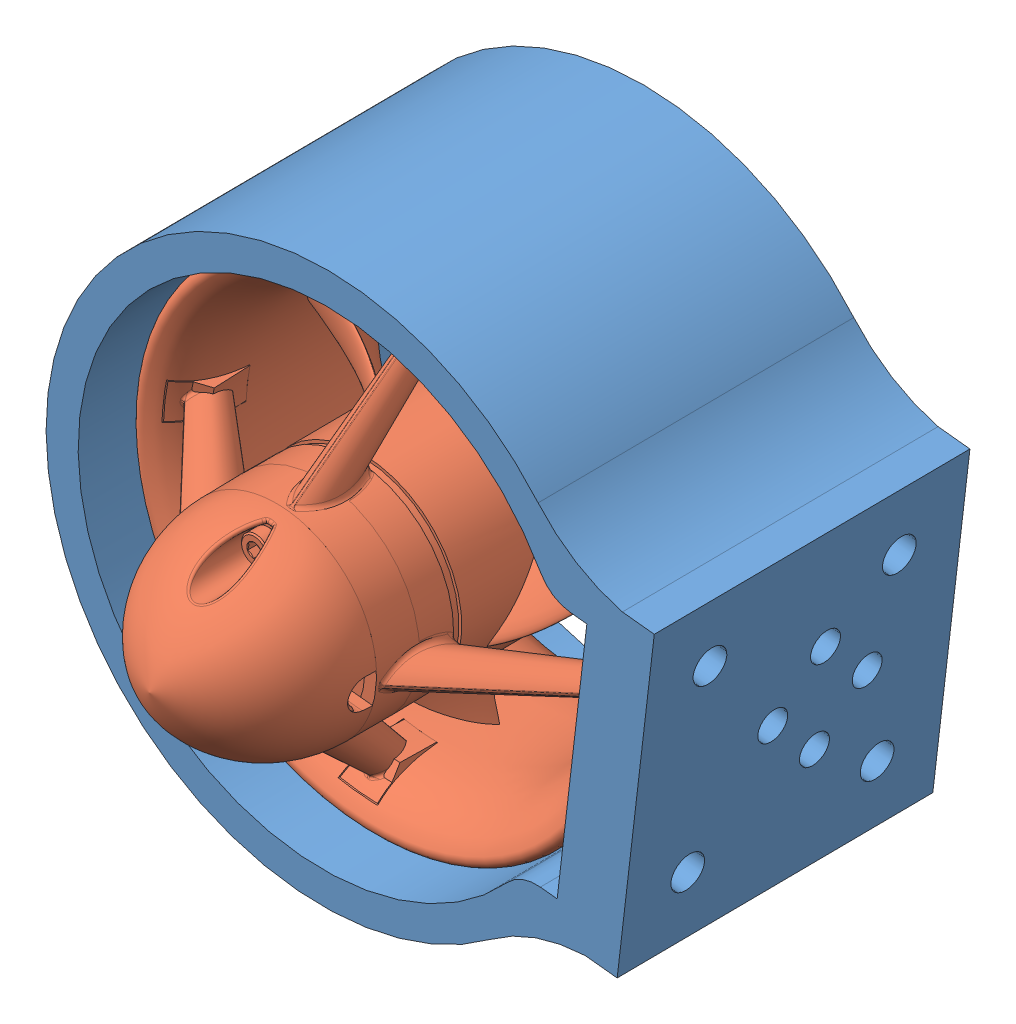
SolidWorks assembly CR-SA-003-HorizontalMotors, configuration Default. Lengths in mm.
Overall size (129.7 123.38 113.5).
2 component instances, 2 part files, 3 mates.
Components (placement in the parent):
- CR-P-0005b-Frame-MotorMount Horizontal-1: CR-P-0005b-Frame-MotorMount Horizontal [Default] at (31.0866 129.8418 39.6539) x (0.993197 -0.116171 -0.007981) z (0.007981 -0.000465 0.999968) size (117.16 110.49 63.5)
- CR-P-0003-T200-THRUSTER-R1-1: CR-P-0003-T200-THRUSTER-R1 [Default] at (31.5506 129.8024 71.3376) x (-0.116171 -0.993229 0.000465) z (0.007981 -0.000465 0.999968) size (96.71 97.53 112.68)
Mates (geometry in assembly coordinates):
- Coincident3: coincident anti-aligned: plane of CR-P-0005b-Frame-MotorMount Horizontal-1 through (80.4711 124.0952 102.7591) normal (-0.993197 0.116171 0.007981); plane of CR-P-0003-T200-THRUSTER-R1-1 through (80.1753 124.1125 65.695) normal (0.993197 -0.116171 -0.007981)
- Concentric1: concentric anti-aligned: circle of CR-P-0005b-Frame-MotorMount Horizontal-1; circle of CR-P-0003-T200-THRUSTER-R1-1
- Concentric2: concentric anti-aligned: circle of CR-P-0005b-Frame-MotorMount Horizontal-1; circle of CR-P-0003-T200-THRUSTER-R1-1
